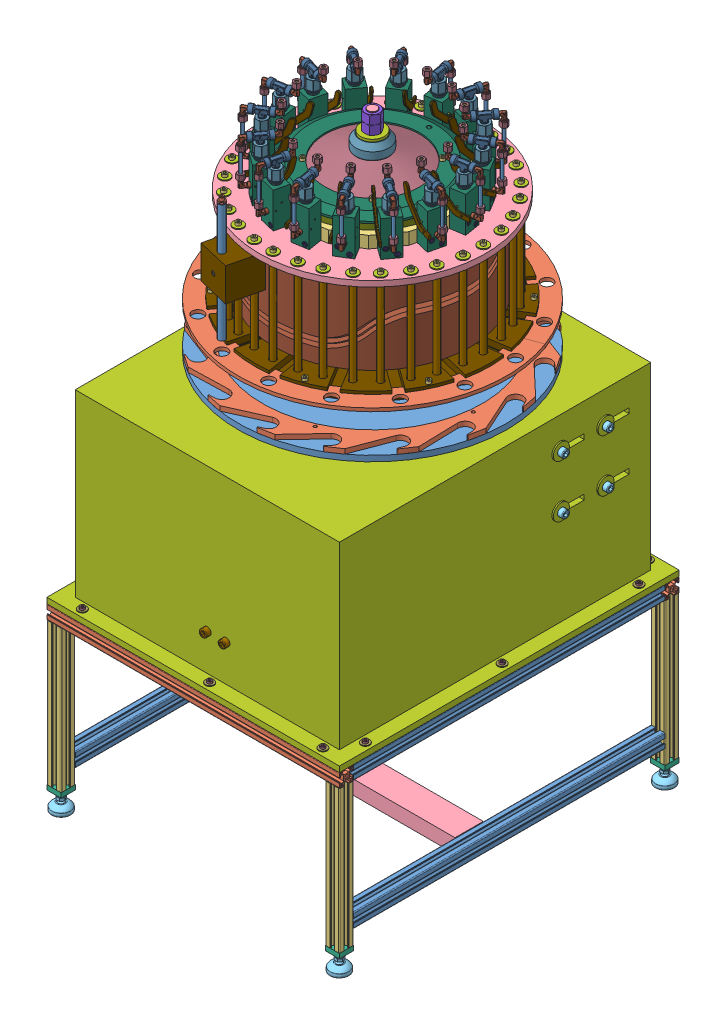
SolidWorks assembly Assieme_FINALE, configuration Default. Lengths in mm. (continued)
Components (placement in the parent): (continued)
- assieme parte rotante-2: assieme parte rotante [Default] at (-8.3038 623.9178 -528.0599) x (0 1 0) z (-0.913062 0 0.407822) size (749.63 778.63 778.63) (continued)
  - M6 16mm-40: M6 16mm [ISO 4762 M6 x 16 - 16N] at (167.0433 -143.7592 568.3922) x (1 0 0) z (0 -0.866025 0.5) size (22 10 10)
  - M6 16mm-41: M6 16mm [ISO 4762 M6 x 16 - 16N] at (167.0433 -72.7177 618.7576) x (1 0 0) z (0 -0.608761 0.793353) size (22 10 10)
  - M6 16mm-42: M6 16mm [ISO 4762 M6 x 16 - 16N] at (167.0433 12.1901 638.1029) x (1 0 0) z (0 -0.258819 0.965926) size (22 10 10)
  - M6 16mm-43: M6 16mm [ISO 4762 M6 x 16 - 16N] at (167.0433 98.0378 623.4827) x (1 0 0) z (0 0.130526 0.991445) size (22 10 10)
  - M6 16mm-44: M6 16mm [ISO 4762 M6 x 16 - 16N] at (167.0433 171.7559 577.1229) x (1 0 0) z (0 0.5 0.866025) size (22 10 10)
  - M6 16mm-45: M6 16mm [ISO 4762 M6 x 16 - 16N] at (167.0433 222.1213 506.0814) x (1 0 0) z (0 0.793353 0.608761) size (22 10 10)
  - M6 16mm-46: M6 16mm [ISO 4762 M6 x 16 - 16N] at (167.0433 241.4666 421.1736) x (1 0 0) z (0 0.965926 0.258819) size (22 10 10)
  - M6 16mm-47: M6 16mm [ISO 4762 M6 x 16 - 16N] at (167.0433 226.8464 335.3259) x (1 0 0) z (0 0.991445 -0.130526) size (22 10 10)
  - M6 16mm-48: M6 16mm [ISO 4762 M6 x 16 - 16N] at (167.0433 180.4866 261.6078) x (1 0 0) z (0 0.866025 -0.5) size (22 10 10)
  - M6 16mm-49: M6 16mm [ISO 4762 M6 x 16 - 16N] at (167.0433 109.4451 211.2424) x (1 0 0) z (0 0.608761 -0.793353) size (22 10 10)
  - asta scorrimento carello-18: asta scorrimento carello [Default] at (287.5433 -61.3104 206.5173) x (0 -0.130526 -0.991445) z (-1 0 0) size (12 12 225)
  - asta scorrimento carello-19: asta scorrimento carello [Default] at (287.5433 -135.0285 252.8771) x (0 -0.5 -0.866025) z (-1 0 0) size (12 12 225)
  - asta scorrimento carello-20: asta scorrimento carello [Default] at (287.5433 -185.3939 323.9186) x (0 -0.793353 -0.608761) z (-1 0 0) size (12 12 225)
  - asta scorrimento carello-21: asta scorrimento carello [Default] at (287.5433 -204.7392 408.8264) x (0 -0.965926 -0.258819) z (-1 0 0) size (12 12 225)
  - asta scorrimento carello-22: asta scorrimento carello [Default] at (287.5433 -190.119 494.6741) x (0 -0.991445 0.130526) z (-1 0 0) size (12 12 225)
  - asta scorrimento carello-23: asta scorrimento carello [Default] at (287.5433 -143.7592 568.3922) x (0 -0.866025 0.5) z (-1 0 0) size (12 12 225)
  - asta scorrimento carello-24: asta scorrimento carello [Default] at (287.5433 -72.7177 618.7576) x (0 -0.608761 0.793353) z (-1 0 0) size (12 12 225)
  - asta scorrimento carello-25: asta scorrimento carello [Default] at (287.5433 12.1901 638.1029) x (0 -0.258819 0.965926) z (-1 0 0) size (12 12 225)
  - asta scorrimento carello-26: asta scorrimento carello [Default] at (287.5433 98.0378 623.4827) x (0 0.130526 0.991445) z (-1 0 0) size (12 12 225)
  - asta scorrimento carello-27: asta scorrimento carello [Default] at (287.5433 171.7559 577.1229) x (0 0.5 0.866025) z (-1 0 0) size (12 12 225)
  - asta scorrimento carello-28: asta scorrimento carello [Default] at (287.5433 222.1213 506.0814) x (0 0.793353 0.608761) z (-1 0 0) size (12 12 225)
  - asta scorrimento carello-29: asta scorrimento carello [Default] at (287.5433 241.4666 421.1736) x (0 0.965926 0.258819) z (-1 0 0) size (12 12 225)
  - asta scorrimento carello-30: asta scorrimento carello [Default] at (287.5433 226.8464 335.3259) x (0 0.991445 -0.130526) z (-1 0 0) size (12 12 225)
  - asta scorrimento carello-31: asta scorrimento carello [Default] at (287.5433 180.4866 261.6078) x (0 0.866025 -0.5) z (-1 0 0) size (12 12 225)
  - asta scorrimento carello-32: asta scorrimento carello [Default] at (287.5433 109.4451 211.2424) x (0 0.608761 -0.793353) z (-1 0 0) size (12 12 225)
  - rondella M6-129: rondella M6 [Washer ISO 7094 - 6] at (400.0433 -61.3104 206.5173) x (-1 0 0) z (0 0.991445 -0.130526) size (2 22 22)
  - rondella M6-130: rondella M6 [Washer ISO 7094 - 6] at (400.0433 -135.0285 252.8771) x (-1 0 0) z (0 0.866025 -0.5) size (2 22 22)
  - rondella M6-131: rondella M6 [Washer ISO 7094 - 6] at (400.0433 -185.3939 323.9186) x (-1 0 0) z (0 0.608761 -0.793353) size (2 22 22)
  - rondella M6-132: rondella M6 [Washer ISO 7094 - 6] at (400.0433 -204.7392 408.8264) x (-1 0 0) z (0 0.258819 -0.965926) size (2 22 22)
  - rondella M6-133: rondella M6 [Washer ISO 7094 - 6] at (400.0433 -190.119 494.6741) x (-1 0 0) z (0 -0.130526 -0.991445) size (2 22 22)
  - rondella M6-134: rondella M6 [Washer ISO 7094 - 6] at (400.0433 -143.7592 568.3922) x (-1 0 0) z (0 -0.5 -0.866025) size (2 22 22)
  - rondella M6-135: rondella M6 [Washer ISO 7094 - 6] at (400.0433 -72.7177 618.7576) x (-1 0 0) z (0 -0.793353 -0.608761) size (2 22 22)
  - rondella M6-136: rondella M6 [Washer ISO 7094 - 6] at (400.0433 12.1901 638.1029) x (-1 0 0) z (0 -0.965926 -0.258819) size (2 22 22)
  - rondella M6-137: rondella M6 [Washer ISO 7094 - 6] at (400.0433 98.0378 623.4827) x (-1 0 0) z (0 -0.991445 0.130526) size (2 22 22)
  - rondella M6-138: rondella M6 [Washer ISO 7094 - 6] at (400.0433 171.7559 577.1229) x (-1 0 0) z (0 -0.866025 0.5) size (2 22 22)
  - rondella M6-139: rondella M6 [Washer ISO 7094 - 6] at (400.0433 222.1213 506.0814) x (-1 0 0) z (0 -0.608761 0.793353) size (2 22 22)
  - rondella M6-140: rondella M6 [Washer ISO 7094 - 6] at (400.0433 241.4666 421.1736) x (-1 0 0) z (0 -0.258819 0.965926) size (2 22 22)
  - rondella M6-141: rondella M6 [Washer ISO 7094 - 6] at (400.0433 226.8464 335.3259) x (-1 0 0) z (0 0.130526 0.991445) size (2 22 22)
  - rondella M6-142: rondella M6 [Washer ISO 7094 - 6] at (400.0433 180.4866 261.6078) x (-1 0 0) z (0 0.5 0.866025) size (2 22 22)
  - rondella M6-143: rondella M6 [Washer ISO 7094 - 6] at (400.0433 109.4451 211.2424) x (-1 0 0) z (0 0.793353 0.608761) size (2 22 22)
  - M6 16mm-50: M6 16mm [ISO 4762 M6 x 16 - 16N] at (408.0433 -61.3104 206.5173) x (-1 0 0) z (0 0.130526 0.991445) size (22 10 10)
  - M6 16mm-51: M6 16mm [ISO 4762 M6 x 16 - 16N] at (408.0433 -135.0285 252.8771) x (-1 0 0) z (0 0.5 0.866025) size (22 10 10)
  - M6 16mm-52: M6 16mm [ISO 4762 M6 x 16 - 16N] at (408.0433 -185.3939 323.9186) x (-1 0 0) z (0 0.793353 0.608761) size (22 10 10)
  - M6 16mm-53: M6 16mm [ISO 4762 M6 x 16 - 16N] at (408.0433 -204.7392 408.8264) x (-1 0 0) z (0 0.965926 0.258819) size (22 10 10)
  - M6 16mm-54: M6 16mm [ISO 4762 M6 x 16 - 16N] at (408.0433 -190.119 494.6741) x (-1 0 0) z (0 0.991445 -0.130526) size (22 10 10)
  - M6 16mm-55: M6 16mm [ISO 4762 M6 x 16 - 16N] at (408.0433 -143.7592 568.3922) x (-1 0 0) z (0 0.866025 -0.5) size (22 10 10)
  - M6 16mm-56: M6 16mm [ISO 4762 M6 x 16 - 16N] at (408.0433 -72.7177 618.7576) x (-1 0 0) z (0 0.608761 -0.793353) size (22 10 10)
  - M6 16mm-57: M6 16mm [ISO 4762 M6 x 16 - 16N] at (408.0433 12.1901 638.1029) x (-1 0 0) z (0 0.258819 -0.965926) size (22 10 10)
  - M6 16mm-58: M6 16mm [ISO 4762 M6 x 16 - 16N] at (408.0433 98.0378 623.4827) x (-1 0 0) z (0 -0.130526 -0.991445) size (22 10 10)
  - M6 16mm-59: M6 16mm [ISO 4762 M6 x 16 - 16N] at (408.0433 171.7559 577.1229) x (-1 0 0) z (0 -0.5 -0.866025) size (22 10 10)
  - M6 16mm-60: M6 16mm [ISO 4762 M6 x 16 - 16N] at (408.0433 222.1213 506.0814) x (-1 0 0) z (0 -0.793353 -0.608761) size (22 10 10)
  - M6 16mm-61: M6 16mm [ISO 4762 M6 x 16 - 16N] at (408.0433 241.4666 421.1736) x (-1 0 0) z (0 -0.965926 -0.258819) size (22 10 10)
  - M6 16mm-62: M6 16mm [ISO 4762 M6 x 16 - 16N] at (408.0433 226.8464 335.3259) x (-1 0 0) z (0 -0.991445 0.130526) size (22 10 10)
  - M6 16mm-63: M6 16mm [ISO 4762 M6 x 16 - 16N] at (408.0433 180.4866 261.6078) x (-1 0 0) z (0 -0.866025 0.5) size (22 10 10)
  - M6 16mm-64: M6 16mm [ISO 4762 M6 x 16 - 16N] at (408.0433 109.4451 211.2424) x (-1 0 0) z (0 -0.608761 0.793353) size (22 10 10)
  - AssiemeValvola-2: AssiemeValvola [Default] at (515.3257 40.5532 246.4544) x (0 -0.130526 0.991445) z (0 0.991445 0.130526) size (90.26 138.63 38)
    - RaccordoT-1: RaccordoT [Default] at origin size (43 29.75 16.5)
    - Raccordo a L-1: Raccordo a L [Default] at (-30 0 0) x (0 -1 0) z (0 0 -1) size (28.34 25.51 14.01)
      - 1809_06_10_01-1: 1809_06_10_01 [Default] at origin size (22.49 23 10)
      - 1809_06_10_02-1: 1809_06_10_02 [Default] at origin size (6.5 8.5 8.5)
      - 1809_06_10_03-1: 1809_06_10_03 [Default] at origin size (11.02 15.01 14.01)
    - Raccordo a L-2: Raccordo a L [Default] at (30 0 0) x (0 1 0) z (0 0 -1) size (28.34 25.51 14.01)
      - 1809_06_10_01-1: 1809_06_10_01 [Default] at origin size (22.49 23 10)
      - 1809_06_10_02-1: 1809_06_10_02 [Default] at origin size (6.5 8.5 8.5)
      - 1809_06_10_03-1: 1809_06_10_03 [Default] at origin size (11.02 15.01 14.01)
    - TappoChiusura-1: TappoChiusura [Default] at (0 -32 0) x (0 -1 0) z (0 0 1) size (38.28 26.74 26.74)
    - CorpoValvola-1: CorpoValvola [Default] at (-15 -115.2824 0) size (30 75 34)
    - Raccordo a L-3: Raccordo a L [Default] at (-30 -88.2824 0) x (0 1 0) z (0 0 1) size (28.34 25.51 14.01)
      - 1809_06_10_01-1: 1809_06_10_01 [Default] at origin size (22.49 23 10)
      - 1809_06_10_02-1: 1809_06_10_02 [Default] at origin size (6.5 8.5 8.5)
      - 1809_06_10_03-1: 1809_06_10_03 [Default] at origin size (11.02 15.01 14.01)
    - Spina_3x38-1: Spina_3x38 [Default] at (0 -68.2824 -21) x (-1 0 0) z (0 0 1) size (3 3 38)
    - Spina_3x38-2: Spina_3x38 [Default] at (-10 -80.2824 -21) x (0.996193 0.087174 0) z (0 0 1) size (3 3 38)
    - M5 40mm-3: M5 40mm [ISO 4762 M5 x 40 - 40N] at (-14.6 -108.7824 9) size (45 8.5 8.5)
    - M5 40mm-2: M5 40mm [ISO 4762 M5 x 40 - 40N] at (-14.6 -96.7824 -9) size (45 8.5 8.5)
    - LevaValvola-1: LevaValvola [Default] at (-24.507 -86.571 -17) x (0.996193 0.087174 0) z (0 0 1) size (77.55 60.2 4)
    - Tubo-1: Tubo [Default] at (-30 -15.9665 0) x (1 0 0) z (0 -1 0) size (6 6 56.4)
  - AssiemeValvola-3: AssiemeValvola [Default] at (515.3257 -25.6355 250.7926) x (0 0.258819 0.965926) z (0 0.965926 -0.258819) size (90.26 138.63 38)
    - RaccordoT-1: RaccordoT [Default] at origin size (43 29.75 16.5)
    - Raccordo a L-1: Raccordo a L [Default] at (-30 0 0) x (0 -1 0) z (0 0 -1) size (28.34 25.51 14.01)
      - 1809_06_10_01-1: 1809_06_10_01 [Default] at origin size (22.49 23 10)
      - 1809_06_10_02-1: 1809_06_10_02 [Default] at origin size (6.5 8.5 8.5)
      - 1809_06_10_03-1: 1809_06_10_03 [Default] at origin size (11.02 15.01 14.01)
    - Raccordo a L-2: Raccordo a L [Default] at (30 0 0) x (0 1 0) z (0 0 -1) size (28.34 25.51 14.01)
      - 1809_06_10_01-1: 1809_06_10_01 [Default] at origin size (22.49 23 10)
      - 1809_06_10_02-1: 1809_06_10_02 [Default] at origin size (6.5 8.5 8.5)
      - 1809_06_10_03-1: 1809_06_10_03 [Default] at origin size (11.02 15.01 14.01)
    - TappoChiusura-1: TappoChiusura [Default] at (0 -32 0) x (0 -1 0) z (0 0 1) size (38.28 26.74 26.74)
    - CorpoValvola-1: CorpoValvola [Default] at (-15 -115.2824 0) size (30 75 34)
    - Raccordo a L-3: Raccordo a L [Default] at (-30 -88.2824 0) x (0 1 0) z (0 0 1) size (28.34 25.51 14.01)
      - 1809_06_10_01-1: 1809_06_10_01 [Default] at origin size (22.49 23 10)
      - 1809_06_10_02-1: 1809_06_10_02 [Default] at origin size (6.5 8.5 8.5)
      - 1809_06_10_03-1: 1809_06_10_03 [Default] at origin size (11.02 15.01 14.01)
    - Spina_3x38-1: Spina_3x38 [Default] at (0 -68.2824 -21) x (-1 0 0) z (0 0 1) size (3 3 38)
    - Spina_3x38-2: Spina_3x38 [Default] at (-10 -80.2824 -21) x (0.996193 0.087174 0) z (0 0 1) size (3 3 38)
    - M5 40mm-3: M5 40mm [ISO 4762 M5 x 40 - 40N] at (-14.6 -108.7824 9) size (45 8.5 8.5)
    - M5 40mm-2: M5 40mm [ISO 4762 M5 x 40 - 40N] at (-14.6 -96.7824 -9) size (45 8.5 8.5)
    - LevaValvola-1: LevaValvola [Default] at (-24.507 -86.571 -17) x (0.996193 0.087174 0) z (0 0 1) size (77.55 60.2 4)
    - Tubo-1: Tubo [Default] at (-30 -15.9665 0) x (1 0 0) z (0 -1 0) size (6 6 56.4)
  - AssiemeValvola-4: AssiemeValvola [Default] at (515.3257 -85.1257 280.1299) x (0 0.608761 0.793353) z (0 0.793353 -0.608761) size (90.26 138.63 38)
    - RaccordoT-1: RaccordoT [Default] at origin size (43 29.75 16.5)
    - Raccordo a L-1: Raccordo a L [Default] at (-30 0 0) x (0 -1 0) z (0 0 -1) size (28.34 25.51 14.01)
      - 1809_06_10_01-1: 1809_06_10_01 [Default] at origin size (22.49 23 10)
      - 1809_06_10_02-1: 1809_06_10_02 [Default] at origin size (6.5 8.5 8.5)
      - 1809_06_10_03-1: 1809_06_10_03 [Default] at origin size (11.02 15.01 14.01)
    - Raccordo a L-2: Raccordo a L [Default] at (30 0 0) x (0 1 0) z (0 0 -1) size (28.34 25.51 14.01)
      - 1809_06_10_01-1: 1809_06_10_01 [Default] at origin size (22.49 23 10)
      - 1809_06_10_02-1: 1809_06_10_02 [Default] at origin size (6.5 8.5 8.5)
      - 1809_06_10_03-1: 1809_06_10_03 [Default] at origin size (11.02 15.01 14.01)
    - TappoChiusura-1: TappoChiusura [Default] at (0 -32 0) x (0 -1 0) z (0 0 1) size (38.28 26.74 26.74)
    - CorpoValvola-1: CorpoValvola [Default] at (-15 -115.2824 0) size (30 75 34)
    - Raccordo a L-3: Raccordo a L [Default] at (-30 -88.2824 0) x (0 1 0) z (0 0 1) size (28.34 25.51 14.01)
      - 1809_06_10_01-1: 1809_06_10_01 [Default] at origin size (22.49 23 10)
      - 1809_06_10_02-1: 1809_06_10_02 [Default] at origin size (6.5 8.5 8.5)
      - 1809_06_10_03-1: 1809_06_10_03 [Default] at origin size (11.02 15.01 14.01)
    - Spina_3x38-1: Spina_3x38 [Default] at (0 -68.2824 -21) x (-1 0 0) z (0 0 1) size (3 3 38)
    - Spina_3x38-2: Spina_3x38 [Default] at (-10 -80.2824 -21) x (0.996193 0.087174 0) z (0 0 1) size (3 3 38)
    - M5 40mm-3: M5 40mm [ISO 4762 M5 x 40 - 40N] at (-14.6 -108.7824 9) size (45 8.5 8.5)
    - M5 40mm-2: M5 40mm [ISO 4762 M5 x 40 - 40N] at (-14.6 -96.7824 -9) size (45 8.5 8.5)
    - LevaValvola-1: LevaValvola [Default] at (-24.507 -86.571 -17) x (0.996193 0.087174 0) z (0 0 1) size (77.55 60.2 4)
    - Tubo-1: Tubo [Default] at (-30 -15.9665 0) x (1 0 0) z (0 -1 0) size (6 6 56.4)
  - AssiemeValvola-5: AssiemeValvola [Default] at (515.3257 -128.8606 330) x (0 0.866025 0.5) z (0 0.5 -0.866025) size (90.26 138.63 38)
    - RaccordoT-1: RaccordoT [Default] at origin size (43 29.75 16.5)
    - Raccordo a L-1: Raccordo a L [Default] at (-30 0 0) x (0 -1 0) z (0 0 -1) size (28.34 25.51 14.01)
      - 1809_06_10_01-1: 1809_06_10_01 [Default] at origin size (22.49 23 10)
      - 1809_06_10_02-1: 1809_06_10_02 [Default] at origin size (6.5 8.5 8.5)
      - 1809_06_10_03-1: 1809_06_10_03 [Default] at origin size (11.02 15.01 14.01)
    - Raccordo a L-2: Raccordo a L [Default] at (30 0 0) x (0 1 0) z (0 0 -1) size (28.34 25.51 14.01)
      - 1809_06_10_01-1: 1809_06_10_01 [Default] at origin size (22.49 23 10)
      - 1809_06_10_02-1: 1809_06_10_02 [Default] at origin size (6.5 8.5 8.5)
      - 1809_06_10_03-1: 1809_06_10_03 [Default] at origin size (11.02 15.01 14.01)
    - TappoChiusura-1: TappoChiusura [Default] at (0 -32 0) x (0 -1 0) z (0 0 1) size (38.28 26.74 26.74)
    - CorpoValvola-1: CorpoValvola [Default] at (-15 -115.2824 0) size (30 75 34)
    - Raccordo a L-3: Raccordo a L [Default] at (-30 -88.2824 0) x (0 1 0) z (0 0 1) size (28.34 25.51 14.01)
      - 1809_06_10_01-1: 1809_06_10_01 [Default] at origin size (22.49 23 10)
      - 1809_06_10_02-1: 1809_06_10_02 [Default] at origin size (6.5 8.5 8.5)
      - 1809_06_10_03-1: 1809_06_10_03 [Default] at origin size (11.02 15.01 14.01)
    - Spina_3x38-1: Spina_3x38 [Default] at (0 -68.2824 -21) x (-1 0 0) z (0 0 1) size (3 3 38)
    - Spina_3x38-2: Spina_3x38 [Default] at (-10 -80.2824 -21) x (0.996193 0.087174 0) z (0 0 1) size (3 3 38)
    - M5 40mm-3: M5 40mm [ISO 4762 M5 x 40 - 40N] at (-14.6 -108.7824 9) size (45 8.5 8.5)
    - M5 40mm-2: M5 40mm [ISO 4762 M5 x 40 - 40N] at (-14.6 -96.7824 -9) size (45 8.5 8.5)
    - LevaValvola-1: LevaValvola [Default] at (-24.507 -86.571 -17) x (0.996193 0.087174 0) z (0 0 1) size (77.55 60.2 4)
    - Tubo-1: Tubo [Default] at (-30 -15.9665 0) x (1 0 0) z (0 -1 0) size (6 6 56.4)
  - AssiemeValvola-6: AssiemeValvola [Default] at (515.3257 -150.1819 392.8105) x (0 0.991445 0.130526) z (0 0.130526 -0.991445) size (90.26 138.63 38)
    - RaccordoT-1: RaccordoT [Default] at origin size (43 29.75 16.5)
    - Raccordo a L-1: Raccordo a L [Default] at (-30 0 0) x (0 -1 0) z (0 0 -1) size (28.34 25.51 14.01)
      - 1809_06_10_01-1: 1809_06_10_01 [Default] at origin size (22.49 23 10)
      - 1809_06_10_02-1: 1809_06_10_02 [Default] at origin size (6.5 8.5 8.5)
      - 1809_06_10_03-1: 1809_06_10_03 [Default] at origin size (11.02 15.01 14.01)
    - Raccordo a L-2: Raccordo a L [Default] at (30 0 0) x (0 1 0) z (0 0 -1) size (28.34 25.51 14.01)
      - 1809_06_10_01-1: 1809_06_10_01 [Default] at origin size (22.49 23 10)
      - 1809_06_10_02-1: 1809_06_10_02 [Default] at origin size (6.5 8.5 8.5)
      - 1809_06_10_03-1: 1809_06_10_03 [Default] at origin size (11.02 15.01 14.01)
    - TappoChiusura-1: TappoChiusura [Default] at (0 -32 0) x (0 -1 0) z (0 0 1) size (38.28 26.74 26.74)
    - CorpoValvola-1: CorpoValvola [Default] at (-15 -115.2824 0) size (30 75 34)
    - Raccordo a L-3: Raccordo a L [Default] at (-30 -88.2824 0) x (0 1 0) z (0 0 1) size (28.34 25.51 14.01)
      - 1809_06_10_01-1: 1809_06_10_01 [Default] at origin size (22.49 23 10)
      - 1809_06_10_02-1: 1809_06_10_02 [Default] at origin size (6.5 8.5 8.5)
      - 1809_06_10_03-1: 1809_06_10_03 [Default] at origin size (11.02 15.01 14.01)
    - Spina_3x38-1: Spina_3x38 [Default] at (0 -68.2824 -21) x (-1 0 0) z (0 0 1) size (3 3 38)
    - Spina_3x38-2: Spina_3x38 [Default] at (-10 -80.2824 -21) x (0.996193 0.087174 0) z (0 0 1) size (3 3 38)
    - M5 40mm-3: M5 40mm [ISO 4762 M5 x 40 - 40N] at (-14.6 -108.7824 9) size (45 8.5 8.5)
    - M5 40mm-2: M5 40mm [ISO 4762 M5 x 40 - 40N] at (-14.6 -96.7824 -9) size (45 8.5 8.5)
    - LevaValvola-1: LevaValvola [Default] at (-24.507 -86.571 -17) x (0.996193 0.087174 0) z (0 0 1) size (77.55 60.2 4)
    - Tubo-1: Tubo [Default] at (-30 -15.9665 0) x (1 0 0) z (0 -1 0) size (6 6 56.4)
  - AssiemeValvola-7: AssiemeValvola [Default] at (515.3257 -145.8437 458.9992) x (0 0.965926 -0.258819) z (0 -0.258819 -0.965926) size (90.26 138.63 38)
    - RaccordoT-1: RaccordoT [Default] at origin size (43 29.75 16.5)
    - Raccordo a L-1: Raccordo a L [Default] at (-30 0 0) x (0 -1 0) z (0 0 -1) size (28.34 25.51 14.01)
      - 1809_06_10_01-1: 1809_06_10_01 [Default] at origin size (22.49 23 10)
      - 1809_06_10_02-1: 1809_06_10_02 [Default] at origin size (6.5 8.5 8.5)
      - 1809_06_10_03-1: 1809_06_10_03 [Default] at origin size (11.02 15.01 14.01)
    - Raccordo a L-2: Raccordo a L [Default] at (30 0 0) x (0 1 0) z (0 0 -1) size (28.34 25.51 14.01)
      - 1809_06_10_01-1: 1809_06_10_01 [Default] at origin size (22.49 23 10)
      - 1809_06_10_02-1: 1809_06_10_02 [Default] at origin size (6.5 8.5 8.5)
      - 1809_06_10_03-1: 1809_06_10_03 [Default] at origin size (11.02 15.01 14.01)
    - TappoChiusura-1: TappoChiusura [Default] at (0 -32 0) x (0 -1 0) z (0 0 1) size (38.28 26.74 26.74)
    - CorpoValvola-1: CorpoValvola [Default] at (-15 -115.2824 0) size (30 75 34)
    - Raccordo a L-3: Raccordo a L [Default] at (-30 -88.2824 0) x (0 1 0) z (0 0 1) size (28.34 25.51 14.01)
      - 1809_06_10_01-1: 1809_06_10_01 [Default] at origin size (22.49 23 10)
      - 1809_06_10_02-1: 1809_06_10_02 [Default] at origin size (6.5 8.5 8.5)
      - 1809_06_10_03-1: 1809_06_10_03 [Default] at origin size (11.02 15.01 14.01)
    - Spina_3x38-1: Spina_3x38 [Default] at (0 -68.2824 -21) x (-1 0 0) z (0 0 1) size (3 3 38)
    - Spina_3x38-2: Spina_3x38 [Default] at (-10 -80.2824 -21) x (0.996193 0.087174 0) z (0 0 1) size (3 3 38)
    - M5 40mm-3: M5 40mm [ISO 4762 M5 x 40 - 40N] at (-14.6 -108.7824 9) size (45 8.5 8.5)
    - M5 40mm-2: M5 40mm [ISO 4762 M5 x 40 - 40N] at (-14.6 -96.7824 -9) size (45 8.5 8.5)
    - LevaValvola-1: LevaValvola [Default] at (-24.507 -86.571 -17) x (0.996193 0.087174 0) z (0 0 1) size (77.55 60.2 4)
    - Tubo-1: Tubo [Default] at (-30 -15.9665 0) x (1 0 0) z (0 -1 0) size (6 6 56.4)
  - AssiemeValvola-8: AssiemeValvola [Default] at (515.3257 -116.5064 518.4894) x (0 0.793353 -0.608761) z (0 -0.608761 -0.793353) size (90.26 138.63 38)
    - RaccordoT-1: RaccordoT [Default] at origin size (43 29.75 16.5)
    - Raccordo a L-1: Raccordo a L [Default] at (-30 0 0) x (0 -1 0) z (0 0 -1) size (28.34 25.51 14.01)
      - 1809_06_10_01-1: 1809_06_10_01 [Default] at origin size (22.49 23 10)
      - 1809_06_10_02-1: 1809_06_10_02 [Default] at origin size (6.5 8.5 8.5)
      - 1809_06_10_03-1: 1809_06_10_03 [Default] at origin size (11.02 15.01 14.01)
    - Raccordo a L-2: Raccordo a L [Default] at (30 0 0) x (0 1 0) z (0 0 -1) size (28.34 25.51 14.01)
      - 1809_06_10_01-1: 1809_06_10_01 [Default] at origin size (22.49 23 10)
      - 1809_06_10_02-1: 1809_06_10_02 [Default] at origin size (6.5 8.5 8.5)
      - 1809_06_10_03-1: 1809_06_10_03 [Default] at origin size (11.02 15.01 14.01)
    - TappoChiusura-1: TappoChiusura [Default] at (0 -32 0) x (0 -1 0) z (0 0 1) size (38.28 26.74 26.74)
    - CorpoValvola-1: CorpoValvola [Default] at (-15 -115.2824 0) size (30 75 34)
    - Raccordo a L-3: Raccordo a L [Default] at (-30 -88.2824 0) x (0 1 0) z (0 0 1) size (28.34 25.51 14.01)
      - 1809_06_10_01-1: 1809_06_10_01 [Default] at origin size (22.49 23 10)
      - 1809_06_10_02-1: 1809_06_10_02 [Default] at origin size (6.5 8.5 8.5)
      - 1809_06_10_03-1: 1809_06_10_03 [Default] at origin size (11.02 15.01 14.01)
    - Spina_3x38-1: Spina_3x38 [Default] at (0 -68.2824 -21) x (-1 0 0) z (0 0 1) size (3 3 38)
    - Spina_3x38-2: Spina_3x38 [Default] at (-10 -80.2824 -21) x (0.996193 0.087174 0) z (0 0 1) size (3 3 38)
    - M5 40mm-3: M5 40mm [ISO 4762 M5 x 40 - 40N] at (-14.6 -108.7824 9) size (45 8.5 8.5)
    - M5 40mm-2: M5 40mm [ISO 4762 M5 x 40 - 40N] at (-14.6 -96.7824 -9) size (45 8.5 8.5)
    - LevaValvola-1: LevaValvola [Default] at (-24.507 -86.571 -17) x (0.996193 0.087174 0) z (0 0 1) size (77.55 60.2 4)
    - Tubo-1: Tubo [Default] at (-30 -15.9665 0) x (1 0 0) z (0 -1 0) size (6 6 56.4)
  - AssiemeValvola-9: AssiemeValvola [Default] at (515.3257 -66.6363 562.2243) x (0 0.5 -0.866025) z (0 -0.866025 -0.5) size (90.26 138.63 38)
    - RaccordoT-1: RaccordoT [Default] at origin size (43 29.75 16.5)
    - Raccordo a L-1: Raccordo a L [Default] at (-30 0 0) x (0 -1 0) z (0 0 -1) size (28.34 25.51 14.01)
      - 1809_06_10_01-1: 1809_06_10_01 [Default] at origin size (22.49 23 10)
      - 1809_06_10_02-1: 1809_06_10_02 [Default] at origin size (6.5 8.5 8.5)
      - 1809_06_10_03-1: 1809_06_10_03 [Default] at origin size (11.02 15.01 14.01)
    - Raccordo a L-2: Raccordo a L [Default] at (30 0 0) x (0 1 0) z (0 0 -1) size (28.34 25.51 14.01)
      - 1809_06_10_01-1: 1809_06_10_01 [Default] at origin size (22.49 23 10)
      - 1809_06_10_02-1: 1809_06_10_02 [Default] at origin size (6.5 8.5 8.5)
      - 1809_06_10_03-1: 1809_06_10_03 [Default] at origin size (11.02 15.01 14.01)
    - TappoChiusura-1: TappoChiusura [Default] at (0 -32 0) x (0 -1 0) z (0 0 1) size (38.28 26.74 26.74)
    - CorpoValvola-1: CorpoValvola [Default] at (-15 -115.2824 0) size (30 75 34)
    - Raccordo a L-3: Raccordo a L [Default] at (-30 -88.2824 0) x (0 1 0) z (0 0 1) size (28.34 25.51 14.01)
      - 1809_06_10_01-1: 1809_06_10_01 [Default] at origin size (22.49 23 10)
      - 1809_06_10_02-1: 1809_06_10_02 [Default] at origin size (6.5 8.5 8.5)
      - 1809_06_10_03-1: 1809_06_10_03 [Default] at origin size (11.02 15.01 14.01)
    - Spina_3x38-1: Spina_3x38 [Default] at (0 -68.2824 -21) x (-1 0 0) z (0 0 1) size (3 3 38)
    - Spina_3x38-2: Spina_3x38 [Default] at (-10 -80.2824 -21) x (0.996193 0.087174 0) z (0 0 1) size (3 3 38)
    - M5 40mm-3: M5 40mm [ISO 4762 M5 x 40 - 40N] at (-14.6 -108.7824 9) size (45 8.5 8.5)
    - M5 40mm-2: M5 40mm [ISO 4762 M5 x 40 - 40N] at (-14.6 -96.7824 -9) size (45 8.5 8.5)
    - LevaValvola-1: LevaValvola [Default] at (-24.507 -86.571 -17) x (0.996193 0.087174 0) z (0 0 1) size (77.55 60.2 4)
    - Tubo-1: Tubo [Default] at (-30 -15.9665 0) x (1 0 0) z (0 -1 0) size (6 6 56.4)
  - AssiemeValvola-10: AssiemeValvola [Default] at (515.3257 -3.8258 583.5456) x (0 0.130526 -0.991445) z (0 -0.991445 -0.130526) size (90.26 138.63 38)
    - RaccordoT-1: RaccordoT [Default] at origin size (43 29.75 16.5)
    - Raccordo a L-1: Raccordo a L [Default] at (-30 0 0) x (0 -1 0) z (0 0 -1) size (28.34 25.51 14.01)
      - 1809_06_10_01-1: 1809_06_10_01 [Default] at origin size (22.49 23 10)
      - 1809_06_10_02-1: 1809_06_10_02 [Default] at origin size (6.5 8.5 8.5)
      - 1809_06_10_03-1: 1809_06_10_03 [Default] at origin size (11.02 15.01 14.01)
    - Raccordo a L-2: Raccordo a L [Default] at (30 0 0) x (0 1 0) z (0 0 -1) size (28.34 25.51 14.01)
      - 1809_06_10_01-1: 1809_06_10_01 [Default] at origin size (22.49 23 10)
      - 1809_06_10_02-1: 1809_06_10_02 [Default] at origin size (6.5 8.5 8.5)
      - 1809_06_10_03-1: 1809_06_10_03 [Default] at origin size (11.02 15.01 14.01)
    - TappoChiusura-1: TappoChiusura [Default] at (0 -32 0) x (0 -1 0) z (0 0 1) size (38.28 26.74 26.74)
    - CorpoValvola-1: CorpoValvola [Default] at (-15 -115.2824 0) size (30 75 34)
    - Raccordo a L-3: Raccordo a L [Default] at (-30 -88.2824 0) x (0 1 0) z (0 0 1) size (28.34 25.51 14.01)
      - 1809_06_10_01-1: 1809_06_10_01 [Default] at origin size (22.49 23 10)
      - 1809_06_10_02-1: 1809_06_10_02 [Default] at origin size (6.5 8.5 8.5)
      - 1809_06_10_03-1: 1809_06_10_03 [Default] at origin size (11.02 15.01 14.01)
    - Spina_3x38-1: Spina_3x38 [Default] at (0 -68.2824 -21) x (-1 0 0) z (0 0 1) size (3 3 38)
    - Spina_3x38-2: Spina_3x38 [Default] at (-10 -80.2824 -21) x (0.996193 0.087174 0) z (0 0 1) size (3 3 38)
    - M5 40mm-3: M5 40mm [ISO 4762 M5 x 40 - 40N] at (-14.6 -108.7824 9) size (45 8.5 8.5)
    - M5 40mm-2: M5 40mm [ISO 4762 M5 x 40 - 40N] at (-14.6 -96.7824 -9) size (45 8.5 8.5)
    - LevaValvola-1: LevaValvola [Default] at (-24.507 -86.571 -17) x (0.996193 0.087174 0) z (0 0 1) size (77.55 60.2 4)
    - Tubo-1: Tubo [Default] at (-30 -15.9665 0) x (1 0 0) z (0 -1 0) size (6 6 56.4)
  - AssiemeValvola-11: AssiemeValvola [Default] at (515.3257 62.3629 579.2074) x (0 -0.258819 -0.965926) z (0 -0.965926 0.258819) size (90.26 138.63 38)
    - RaccordoT-1: RaccordoT [Default] at origin size (43 29.75 16.5)
    - Raccordo a L-1: Raccordo a L [Default] at (-30 0 0) x (0 -1 0) z (0 0 -1) size (28.34 25.51 14.01)
      - 1809_06_10_01-1: 1809_06_10_01 [Default] at origin size (22.49 23 10)
      - 1809_06_10_02-1: 1809_06_10_02 [Default] at origin size (6.5 8.5 8.5)
      - 1809_06_10_03-1: 1809_06_10_03 [Default] at origin size (11.02 15.01 14.01)
    - Raccordo a L-2: Raccordo a L [Default] at (30 0 0) x (0 1 0) z (0 0 -1) size (28.34 25.51 14.01)
      - 1809_06_10_01-1: 1809_06_10_01 [Default] at origin size (22.49 23 10)
      - 1809_06_10_02-1: 1809_06_10_02 [Default] at origin size (6.5 8.5 8.5)
      - 1809_06_10_03-1: 1809_06_10_03 [Default] at origin size (11.02 15.01 14.01)
    - TappoChiusura-1: TappoChiusura [Default] at (0 -32 0) x (0 -1 0) z (0 0 1) size (38.28 26.74 26.74)
    - CorpoValvola-1: CorpoValvola [Default] at (-15 -115.2824 0) size (30 75 34)
    - Raccordo a L-3: Raccordo a L [Default] at (-30 -88.2824 0) x (0 1 0) z (0 0 1) size (28.34 25.51 14.01)
      - 1809_06_10_01-1: 1809_06_10_01 [Default] at origin size (22.49 23 10)
      - 1809_06_10_02-1: 1809_06_10_02 [Default] at origin size (6.5 8.5 8.5)
      - 1809_06_10_03-1: 1809_06_10_03 [Default] at origin size (11.02 15.01 14.01)
    - Spina_3x38-1: Spina_3x38 [Default] at (0 -68.2824 -21) x (-1 0 0) z (0 0 1) size (3 3 38)
    - Spina_3x38-2: Spina_3x38 [Default] at (-10 -80.2824 -21) x (0.996193 0.087174 0) z (0 0 1) size (3 3 38)
    - M5 40mm-3: M5 40mm [ISO 4762 M5 x 40 - 40N] at (-14.6 -108.7824 9) size (45 8.5 8.5)
    - M5 40mm-2: M5 40mm [ISO 4762 M5 x 40 - 40N] at (-14.6 -96.7824 -9) size (45 8.5 8.5)
    - LevaValvola-1: LevaValvola [Default] at (-24.507 -86.571 -17) x (0.996193 0.087174 0) z (0 0 1) size (77.55 60.2 4)
    - Tubo-1: Tubo [Default] at (-30 -15.9665 0) x (1 0 0) z (0 -1 0) size (6 6 56.4)
  - AssiemeValvola-12: AssiemeValvola [Default] at (515.3257 121.8531 549.8701) x (0 -0.608761 -0.793353) z (0 -0.793353 0.608761) size (90.26 138.63 38)
    - RaccordoT-1: RaccordoT [Default] at origin size (43 29.75 16.5)
    - Raccordo a L-1: Raccordo a L [Default] at (-30 0 0) x (0 -1 0) z (0 0 -1) size (28.34 25.51 14.01)
      - 1809_06_10_01-1: 1809_06_10_01 [Default] at origin size (22.49 23 10)
      - 1809_06_10_02-1: 1809_06_10_02 [Default] at origin size (6.5 8.5 8.5)
      - 1809_06_10_03-1: 1809_06_10_03 [Default] at origin size (11.02 15.01 14.01)
    - Raccordo a L-2: Raccordo a L [Default] at (30 0 0) x (0 1 0) z (0 0 -1) size (28.34 25.51 14.01)
      - 1809_06_10_01-1: 1809_06_10_01 [Default] at origin size (22.49 23 10)
      - 1809_06_10_02-1: 1809_06_10_02 [Default] at origin size (6.5 8.5 8.5)
      - 1809_06_10_03-1: 1809_06_10_03 [Default] at origin size (11.02 15.01 14.01)
    - TappoChiusura-1: TappoChiusura [Default] at (0 -32 0) x (0 -1 0) z (0 0 1) size (38.28 26.74 26.74)
    - CorpoValvola-1: CorpoValvola [Default] at (-15 -115.2824 0) size (30 75 34)
    - Raccordo a L-3: Raccordo a L [Default] at (-30 -88.2824 0) x (0 1 0) z (0 0 1) size (28.34 25.51 14.01)
      - 1809_06_10_01-1: 1809_06_10_01 [Default] at origin size (22.49 23 10)
      - 1809_06_10_02-1: 1809_06_10_02 [Default] at origin size (6.5 8.5 8.5)
      - 1809_06_10_03-1: 1809_06_10_03 [Default] at origin size (11.02 15.01 14.01)
    - Spina_3x38-1: Spina_3x38 [Default] at (0 -68.2824 -21) x (-1 0 0) z (0 0 1) size (3 3 38)
    - Spina_3x38-2: Spina_3x38 [Default] at (-10 -80.2824 -21) x (0.996193 0.087174 0) z (0 0 1) size (3 3 38)
    - M5 40mm-3: M5 40mm [ISO 4762 M5 x 40 - 40N] at (-14.6 -108.7824 9) size (45 8.5 8.5)
    - M5 40mm-2: M5 40mm [ISO 4762 M5 x 40 - 40N] at (-14.6 -96.7824 -9) size (45 8.5 8.5)
    - LevaValvola-1: LevaValvola [Default] at (-24.507 -86.571 -17) x (0.996193 0.087174 0) z (0 0 1) size (77.55 60.2 4)
    - Tubo-1: Tubo [Default] at (-30 -15.9665 0) x (1 0 0) z (0 -1 0) size (6 6 56.4)
  - AssiemeValvola-13: AssiemeValvola [Default] at (515.3257 165.588 500) x (0 -0.866025 -0.5) z (0 -0.5 0.866025) size (90.26 138.63 38)
    - RaccordoT-1: RaccordoT [Default] at origin size (43 29.75 16.5)
    - Raccordo a L-1: Raccordo a L [Default] at (-30 0 0) x (0 -1 0) z (0 0 -1) size (28.34 25.51 14.01)
      - 1809_06_10_01-1: 1809_06_10_01 [Default] at origin size (22.49 23 10)
      - 1809_06_10_02-1: 1809_06_10_02 [Default] at origin size (6.5 8.5 8.5)
      - 1809_06_10_03-1: 1809_06_10_03 [Default] at origin size (11.02 15.01 14.01)
    - Raccordo a L-2: Raccordo a L [Default] at (30 0 0) x (0 1 0) z (0 0 -1) size (28.34 25.51 14.01)
      - 1809_06_10_01-1: 1809_06_10_01 [Default] at origin size (22.49 23 10)
      - 1809_06_10_02-1: 1809_06_10_02 [Default] at origin size (6.5 8.5 8.5)
      - 1809_06_10_03-1: 1809_06_10_03 [Default] at origin size (11.02 15.01 14.01)
    - TappoChiusura-1: TappoChiusura [Default] at (0 -32 0) x (0 -1 0) z (0 0 1) size (38.28 26.74 26.74)
    - CorpoValvola-1: CorpoValvola [Default] at (-15 -115.2824 0) size (30 75 34)
    - Raccordo a L-3: Raccordo a L [Default] at (-30 -88.2824 0) x (0 1 0) z (0 0 1) size (28.34 25.51 14.01)
      - 1809_06_10_01-1: 1809_06_10_01 [Default] at origin size (22.49 23 10)
      - 1809_06_10_02-1: 1809_06_10_02 [Default] at origin size (6.5 8.5 8.5)
      - 1809_06_10_03-1: 1809_06_10_03 [Default] at origin size (11.02 15.01 14.01)
    - Spina_3x38-1: Spina_3x38 [Default] at (0 -68.2824 -21) x (-1 0 0) z (0 0 1) size (3 3 38)
    - Spina_3x38-2: Spina_3x38 [Default] at (-10 -80.2824 -21) x (0.996193 0.087174 0) z (0 0 1) size (3 3 38)
    - M5 40mm-3: M5 40mm [ISO 4762 M5 x 40 - 40N] at (-14.6 -108.7824 9) size (45 8.5 8.5)
    - M5 40mm-2: M5 40mm [ISO 4762 M5 x 40 - 40N] at (-14.6 -96.7824 -9) size (45 8.5 8.5)
    - LevaValvola-1: LevaValvola [Default] at (-24.507 -86.571 -17) x (0.996193 0.087174 0) z (0 0 1) size (77.55 60.2 4)
    - Tubo-1: Tubo [Default] at (-30 -15.9665 0) x (1 0 0) z (0 -1 0) size (6 6 56.4)
  - AssiemeValvola-14: AssiemeValvola [Default] at (515.3257 186.9093 437.1895) x (0 -0.991445 -0.130526) z (0 -0.130526 0.991445) size (90.26 138.63 38)
    - RaccordoT-1: RaccordoT [Default] at origin size (43 29.75 16.5)
    - Raccordo a L-1: Raccordo a L [Default] at (-30 0 0) x (0 -1 0) z (0 0 -1) size (28.34 25.51 14.01)
      - 1809_06_10_01-1: 1809_06_10_01 [Default] at origin size (22.49 23 10)
      - 1809_06_10_02-1: 1809_06_10_02 [Default] at origin size (6.5 8.5 8.5)
      - 1809_06_10_03-1: 1809_06_10_03 [Default] at origin size (11.02 15.01 14.01)
    - Raccordo a L-2: Raccordo a L [Default] at (30 0 0) x (0 1 0) z (0 0 -1) size (28.34 25.51 14.01)
      - 1809_06_10_01-1: 1809_06_10_01 [Default] at origin size (22.49 23 10)
      - 1809_06_10_02-1: 1809_06_10_02 [Default] at origin size (6.5 8.5 8.5)
      - 1809_06_10_03-1: 1809_06_10_03 [Default] at origin size (11.02 15.01 14.01)
    - TappoChiusura-1: TappoChiusura [Default] at (0 -32 0) x (0 -1 0) z (0 0 1) size (38.28 26.74 26.74)
    - CorpoValvola-1: CorpoValvola [Default] at (-15 -115.2824 0) size (30 75 34)
    - Raccordo a L-3: Raccordo a L [Default] at (-30 -88.2824 0) x (0 1 0) z (0 0 1) size (28.34 25.51 14.01)
      - 1809_06_10_01-1: 1809_06_10_01 [Default] at origin size (22.49 23 10)
      - 1809_06_10_02-1: 1809_06_10_02 [Default] at origin size (6.5 8.5 8.5)
      - 1809_06_10_03-1: 1809_06_10_03 [Default] at origin size (11.02 15.01 14.01)
    - Spina_3x38-1: Spina_3x38 [Default] at (0 -68.2824 -21) x (-1 0 0) z (0 0 1) size (3 3 38)
    - Spina_3x38-2: Spina_3x38 [Default] at (-10 -80.2824 -21) x (0.996193 0.087174 0) z (0 0 1) size (3 3 38)
    - M5 40mm-3: M5 40mm [ISO 4762 M5 x 40 - 40N] at (-14.6 -108.7824 9) size (45 8.5 8.5)
    - M5 40mm-2: M5 40mm [ISO 4762 M5 x 40 - 40N] at (-14.6 -96.7824 -9) size (45 8.5 8.5)
    - LevaValvola-1: LevaValvola [Default] at (-24.507 -86.571 -17) x (0.996193 0.087174 0) z (0 0 1) size (77.55 60.2 4)
    - Tubo-1: Tubo [Default] at (-30 -15.9665 0) x (1 0 0) z (0 -1 0) size (6 6 56.4)
